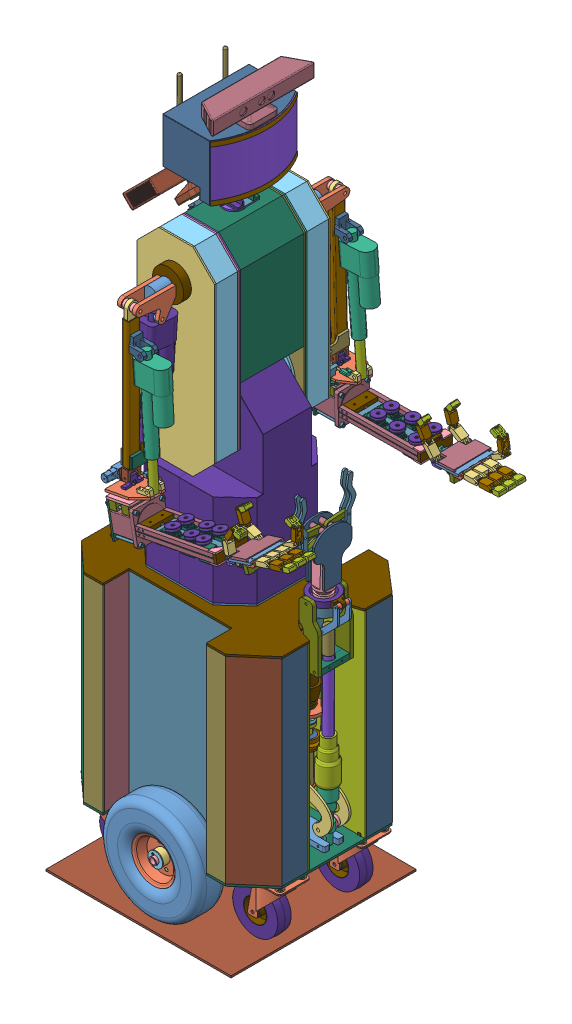
SolidWorks assembly sorbot, configuration По умолчанию. Lengths in mm. (continued)
Mates (geometry in assembly coordinates): (continued)
- Концентричный555: concentric anti-aligned: cylinder of arm.drive.p3-2 through (-20.8275 1162.0905 -207.3595) axis (0 0 -1) radius 6; cylinder of arm.drive.p6-2 through (-20.8275 1162.0905 -222.3595) axis (0 0 1) radius 7
- Заблокировать505: lock: unknown of body.frame.p1-3; unknown of ?
- Заблокировать506: lock: unknown of body.frame.p1-left-1; unknown of ?
- Заблокировать507: lock: unknown of body.frame.p1-3; unknown of ?
- Заблокировать508: lock: unknown of body.frame.p1-3; unknown of arm.drive.p6-1
- Заблокировать510: lock: unknown of ?; unknown of ?
- Концентричный559: concentric anti-aligned: cylinder of arm.drive.p3-2 through (-20.8275 1162.0905 -207.3595) axis (0 0 -1) radius 6; cylinder of m14.nut-1 through (-20.8275 1162.0905 -128.9852) axis (0 0 1) radius 7
- Совпадение1034: coincident anti-aligned: plane of arm.drive.p7-2 through (-42.4721 1162.0905 -109.4852) normal (0 1 0); plane of arm.drive.p7-3 through (-42.4721 1162.0905 -137.4852) normal (0 -1 0)
- Совпадение1035: coincident aligned: plane of arm.drive.p7-2 through (12.3724 1162.0905 -109.4852) normal (0 0 1); plane of arm.drive.p7-3 through (12.3724 1162.0905 -109.4852) normal (0 0 1)
- Совпадение1036: coincident aligned: plane of arm.drive.p7-2 through (-42.4721 1162.0905 -137.4852) normal (-1 0 0); plane of arm.drive.p7-3 through (-42.4721 1162.0905 -109.4852) normal (-1 0 0)
- Концентричный560: concentric anti-aligned: cylinder of arm.drive.p2-pair-1 through (10.8018 1164.5905 -123.4852) axis (0 -1 0) radius 2.5; cylinder of arm.drive.p7-3 through (10.8018 1162.0905 -123.4852) axis (0 1 0) radius 2.5
- Совпадение1038: coincident anti-aligned: plane of m14.nut-1 through (-8.1258 1162.0905 -128.9852) normal (0 0 -1); plane of arm.drive.p7-3 through (-33.7738 1162.0905 -128.9852) normal (0 0 1)
- Заблокировать511: lock: unknown of ?; unknown of ?
- Совпадение1040: coincident anti-aligned: plane of arm.drive.p7-4 through (-9.0342 1232.7974 -150.3) normal (0 1 0); plane of m14.nut-2 through (-2.5764 1232.7974 -139.8) normal (0 -1 0)
- Совпадение1041: coincident anti-aligned: plane of m14.nut-2 through (-2.5764 1254.7974 -150.3) normal (0 0 -1); plane of arm.drive.p7-4 through (-9.0341 1243.9206 -150.3) normal (0 0 1)
- Совпадение1042: coincident: plane of arm.drive.p7-4 through (16.4762 1232.7974 -150.3) normal (-1 0 0); line of m14.nut-2 through (16.4762 1243.7974 -140.8) axis (0 0 -1)
- Заблокировать512: lock: unknown of ?; unknown of ?
- Концентричный562: concentric anti-aligned: cylinder of m14.nut-2 through (3.7745 1243.7974 -139.8) axis (0 0 -1) radius 7; cylinder of arm.drive.p3-1 through (3.7745 1243.7974 -65.7442) axis (0 0 1) radius 6
- Совпадение1043: coincident anti-aligned: plane of arm.drive.p7-5 through (-17.7325 1243.9206 -159.3) normal (0 -1 0); plane of arm.drive.p7-4 through (-17.7325 1243.9206 -131.3) normal (0 1 0)
- Концентричный563: concentric anti-aligned: cylinder of arm.drive.p7-4 through (35.5414 1243.9206 -145.3) axis (0 -1 0) radius 2.5; cylinder of arm.drive.p7-5 through (35.5414 1243.9206 -145.3) axis (0 1 0) radius 2.5
- Совпадение1045: coincident aligned: plane of arm.drive.p7-4 through (-17.7325 1243.9206 -159.3) normal (-1 0 0); plane of arm.drive.p7-5 through (-17.7325 1243.9206 -131.3) normal (-1 0 0)
- Совпадение1046: coincident aligned: plane of arm.drive.p7-4 through (37.112 1243.9206 -131.3) normal (0 0 1); plane of arm.drive.p7-5 through (37.112 1243.9206 -131.3) normal (0 0 1)
- Концентричный564: concentric anti-aligned: cylinder of arm.drive.p2-1 through (35.5414 1246.2974 -145.3) axis (0 -1 0) radius 2.5; cylinder of arm.drive.p7-5 through (35.5414 1243.9206 -145.3) axis (0 1 0) radius 2.5
- Совпадение1047: coincident anti-aligned: plane of body.frame.p4-4 through (-117.3772 1436.2936 -230.3595) normal (0 0 -1); plane of arm.drive.p1.m1-1 through (28.6519 1174.5905 -230.3595) normal (0 0 1)
- Совпадение1048: coincident anti-aligned: plane of body.frame.p4-4 through (-117.3772 1436.2936 -230.3595) normal (0 0 -1); plane of arm.drive.p1.m1-2 through (28.6519 1159.5905 -230.3595) normal (0 0 1)
- Параллельность203: parallel anti-aligned: plane of arm.drive.p1.m1-1 through (28.6519 1164.5905 -234.3595) normal (0 -1 0); plane of arm.drive.p1.m1-2 through (28.6519 1159.5905 -234.3595) normal (0 1 0)
- Совпадение1051: coincident anti-aligned: plane of ? through (48.6519 1164.5905 -237.3595) normal (0 1 0); plane of arm.drive.p1.m1-1 through (28.6519 1164.5905 -234.3595) normal (0 -1 0)
- Совпадение1052: coincident aligned: plane of arm.drive.p1.m1-1 through (68.6519 1174.5904 -230.3595) normal (1 0 0); plane of arm.drive.p1.m1-2 through (68.6519 1159.5904 -230.3595) normal (1 0 0)
- Совпадение1053: coincident anti-aligned: plane of ? through (48.6519 1159.5905 -237.3595) normal (0 -1 0); plane of arm.drive.p1.m1-2 through (28.6519 1159.5905 -234.3595) normal (0 1 0)
- Заблокировать513: lock: unknown of ?; unknown of ?
- Заблокировать514: lock: unknown of ?; unknown of ?
- Концентричный565: concentric aligned: cylinder of ? through (48.6519 1164.5905 -237.3595) axis (0 -1 0) radius 2.5; cylinder of arm.drive.p1.m1-2 through (48.6519 1159.5905 -237.3595) axis (0 -1 0) radius 2.5
- Концентричный566: concentric anti-aligned: cylinder of shoulder.bearing.housing-3 through (-12.6499 1335.3853 -313.3595) axis (0 0 1) radius 15.5; cylinder of body.frame.p4.external-1 through (-12.6499 1335.3853 -288.3595) axis (0 0 -1) radius 21
- Заблокировать516: lock: unknown of ?; unknown of ?
- Заблокировать517: lock: unknown of ?; unknown of ?
- Заблокировать518: lock: unknown of ?; unknown of ?
- Концентричный567: concentric aligned: cylinder of shoulder.bearing.housing-1 through (-12.7629 1335.3853 40.2558) axis (0 0 -1) radius 15.5; cylinder of body.frame.p4.external-2 through (-12.7629 1335.3853 19.2558) axis (0 0 -1) radius 21
- Заблокировать520: lock: unknown of body.frame.p5-1; unknown of body.frame.p4.external-2
- Заблокировать522: lock: unknown of arm.lift.actuator.fixture.p3-1; unknown of body.frame.p4.external-2
- Заблокировать523: lock: unknown of shoulder.bearing.housing-1; unknown of body.frame.p4.external-2
- Заблокировать524: lock: unknown of arm.lift.actuator.fixture.p2-1; unknown of arm.lift.actuator.fixture.p3-1
- Совпадение1061: coincident anti-aligned: plane of ? through (45.4163 1246.2974 -35.7442) normal (0 1 0); plane of arm.drive.p1.m1-4 through (65.4163 1246.2974 -38.7442) normal (0 -1 0)
- Совпадение1064: coincident aligned: plane of arm.drive.p1.m1-3 through (65.4163 1241.2974 -42.7442) normal (1 0 0); plane of arm.drive.p1.m1-4 through (65.4163 1256.2974 -42.7442) normal (1 0 0)
- Совпадение1065: coincident anti-aligned: plane of ? through (45.4163 1241.2974 -35.7442) normal (0 -1 0); plane of arm.drive.p1.m1-3 through (65.4163 1241.2974 -38.7442) normal (0 1 0)
- Концентричный568: concentric aligned: cylinder of ? through (45.4163 1246.2974 -35.7442) axis (0 -1 0) radius 2.5; cylinder of arm.drive.p1.m1-4 through (45.4163 1256.2974 -35.7442) axis (0 -1 0) radius 2.5
- Концентричный569: concentric anti-aligned: cylinder of shoulder.bearing.housing-2 through (-12.4903 1335.516 -67.7442) axis (0 0 1) radius 15.5; cylinder of body.frame.p4.right-1 through (-12.4903 1335.516 -42.7442) axis (0 0 -1) radius 12.5
- Заблокировать527: lock: unknown of arm.lift.actuator.fixture.p3-2; unknown of body.frame.p4.right-1
- Заблокировать528: lock: unknown of shoulder.bearing.housing-2; unknown of body.frame.p4.right-1
- Заблокировать529: lock: unknown of body.frame.p5-1; unknown of body.frame.p4.right-1
- Заблокировать530: lock: unknown of arm.drive.p1.m1-4; unknown of body.frame.p4.right-1
- Заблокировать531: lock: unknown of arm.drive.p1.m1-3; unknown of body.frame.p4.right-1
- Совпадение1067: coincident anti-aligned: plane of body.frame.p1-3 through (92.5097 1436.2936 -46.7442) normal (0 0 1); plane of body.frame.p4.right-1 through (-117.4903 1436.2936 -46.7442) normal (0 0 -1)
- Совпадение1026: coincident anti-aligned: plane of body.frame.p4-4 through (-117.3772 1436.2936 -226.3595) normal (0 0 1); plane of body.frame.p1-left-1 through (92.5148 1436.2936 -226.3595) normal (0 0 -1)
- Концентричный570: concentric aligned: cylinder of arm.drive.motor-1 through (-20.8275 1162.0905 -80.2442) axis (0 0 1) radius 8; cylinder of arm.drive.p8-1 through (-20.8275 1162.0905 -80.2442) axis (0 0 1) radius 8
- Совпадение1069: coincident anti-aligned: plane of arm.drive.motor-1 through (-20.8275 1162.0905 -72.7442) normal (0 0 -1); plane of arm.drive.p8-1 through (-20.8275 1162.0905 -72.7442) normal (0 0 1)
- Концентричный571: concentric aligned: cylinder of arm.drive.motor.pair-1 through (3.7745 1243.7974 -192.8595) axis (0 0 -1) radius 8; cylinder of arm.drive.p8-2 through (3.7745 1243.7974 -192.8595) axis (0 0 -1) radius 8
- Совпадение1070: coincident anti-aligned: plane of arm.drive.motor.pair-1 through (3.7745 1243.7974 -200.3595) normal (0 0 1); plane of arm.drive.p8-2 through (3.7745 1243.7974 -200.3595) normal (0 0 -1)
- Концентричный572: concentric aligned: cylinder of man1.drive1-1 through (-119.3768 773.978 -141.6211) axis (0 -1 0) radius 6; cylinder of tilt.thread.rod.fixture.2-1 through (-119.3768 819.5591 -141.6211) axis (0 -1 0) radius 12
- Совпадение1071: coincident anti-aligned: plane of turret.table-1 through (-20.0648 612.7934 -360.2969) normal (0 1 0); plane of body.tilit.planetary.drive.fixture.p1-1 through (-119.3768 612.7934 -141.6211) normal (0 -1 0)
- Концентричный573: concentric aligned: cylinder of man1.drive1-1 through (-119.3768 703.728 -141.6211) axis (0 -1 0) radius 19; cylinder of body.tilit.planetary.drive.fixture.p1-1 through (-119.3768 622.7934 -141.6211) axis (0 -1 0) radius 42.5
- Заблокировать532: lock: unknown of ?; unknown of ?
- Совпадение1072: coincident anti-aligned: plane of body.tilit.planetary.drive.fixture.p1-1 through (-119.3768 622.7934 -141.6211) normal (0 1 0); plane of body.tilit.planetary.drive.fixture.p2-1 through (-119.3768 622.7934 -141.6211) normal (0 -1 0)
- Концентричный575: concentric aligned: cylinder of body.tilit.planetary.drive.fixture.p1-1 through (-119.3768 622.7934 -141.6211) axis (0 -1 0) radius 42.5; cylinder of body.tilit.planetary.drive.fixture.p2-1 through (-119.3768 626.7934 -141.6211) axis (0 -1 0) radius 42.5
- Концентричный577: concentric aligned: cylinder of man1.drive1-1 through (-119.3768 773.978 -141.6211) axis (0 -1 0) radius 6; cylinder of tilt.thread.rod.fixture.2-2 through (-119.3768 792.5591 -141.6211) axis (0 -1 0) radius 8
- Совпадение1073: coincident anti-aligned: plane of tilt.thread.rod.fixture.2-1 through (-119.3768 793.5591 -141.6211) normal (0 -1 0); plane of tilt.thread.rod.fixture.2-2 through (-119.3768 793.5591 -141.6211) normal (0 1 0)
- Концентричный578: concentric aligned: cylinder of man1.drive1-1 through (-119.3768 703.728 -141.6211) axis (0 -1 0) radius 19; cylinder of body.tilit.planetary.drive.fixture.p3-1 through (-119.3768 703.728 -141.6211) axis (0 -1 0) radius 19
- Совпадение1074: coincident anti-aligned: plane of man1.drive1-1 through (-119.3768 703.728 -141.6211) normal (0 -1 0); plane of body.tilit.planetary.drive.fixture.p3-1 through (-119.3768 703.728 -141.6211) normal (0 1 0)
- Концентричный579: concentric aligned: cylinder of man1.drive1-1 through (-119.3768 761.728 -141.6211) axis (0 -1 0) radius 14.75; cylinder of body.tilit.planetary.drive.fixture.p4-1 through (-119.3768 762.9526 -141.6211) axis (0 -1 0) radius 14.8
- Заблокировать533: lock: unknown of ?; unknown of ?
- Концентричный580: concentric anti-aligned: cylinder of body.tilit.planetary.drive.fixture.p3-1 through (-148.8664 695.728 -141.6211) axis (0 1 0) radius 2.5; cylinder of body.tilit.planetary.drive.fixture.p5-1 through (-148.8664 769.7934 -141.6211) axis (0 -1 0) radius 2.5
- Совпадение1076: coincident aligned: plane of body.tilit.planetary.drive.fixture.p1-1 through (-119.3768 612.7934 -141.6211) normal (0 -1 0); plane of body.tilit.planetary.drive.fixture.p5-1 through (-148.8664 612.7934 -141.6211) normal (0 -1 0)
- Совпадение1077: coincident anti-aligned: plane of body.tilit.planetary.drive.fixture.p1-1 through (-148.8664 618.7934 -141.6211) normal (0 -1 0); plane of m6.nut-13 through (-148.8664 618.7934 -135.8476) normal (0 1 0)
- Концентричный581: concentric aligned: cylinder of body.tilit.planetary.drive.fixture.p5-1 through (-148.8664 769.7934 -141.6211) axis (0 -1 0) radius 2.5; cylinder of m6.nut-13 through (-148.8664 618.7934 -141.6211) axis (0 -1 0) radius 3
- Концентричный582: concentric aligned: cylinder of body.tilit.planetary.drive.fixture.p1-1 through (-119.3768 624.7934 -112.1315) axis (0 -1 0) radius 2.5; cylinder of body.tilit.planetary.drive.fixture.p5-3 through (-119.3768 769.7934 -112.1315) axis (0 -1 0) radius 2.5
- Концентричный583: concentric aligned: cylinder of body.tilit.planetary.drive.fixture.p1-1 through (-89.8872 624.7934 -141.6211) axis (0 -1 0) radius 2.5; cylinder of body.tilit.planetary.drive.fixture.p5-2 through (-89.8872 769.7934 -141.6211) axis (0 -1 0) radius 2.5
- Концентричный584: concentric aligned: cylinder of body.tilit.planetary.drive.fixture.p1-1 through (-119.3768 624.7934 -171.1107) axis (0 -1 0) radius 2.5; cylinder of body.tilit.planetary.drive.fixture.p5-4 through (-119.3768 769.7934 -171.1107) axis (0 -1 0) radius 2.5
- Совпадение1078: coincident aligned: plane of body.tilit.planetary.drive.fixture.p1-1 through (-119.3768 612.7934 -141.6211) normal (0 -1 0); plane of body.tilit.planetary.drive.fixture.p5-4 through (-119.3768 612.7934 -171.1107) normal (0 -1 0)
- Совпадение1079: coincident aligned: plane of body.tilit.planetary.drive.fixture.p1-1 through (-119.3768 612.7934 -141.6211) normal (0 -1 0); plane of body.tilit.planetary.drive.fixture.p5-3 through (-119.3768 612.7934 -112.1315) normal (0 -1 0)
- Совпадение1080: coincident aligned: plane of body.tilit.planetary.drive.fixture.p1-1 through (-119.3768 612.7934 -141.6211) normal (0 -1 0); plane of body.tilit.planetary.drive.fixture.p5-2 through (-89.8872 612.7934 -141.6211) normal (0 -1 0)
- Концентричный585: concentric aligned: cylinder of body.tilit.planetary.drive.fixture.p5-4 through (-119.3768 769.7934 -171.1107) axis (0 -1 0) radius 2.5; cylinder of m6.nut-15 through (-119.3768 618.7934 -171.1107) axis (0 -1 0) radius 3
- Концентричный586: concentric aligned: cylinder of body.tilit.planetary.drive.fixture.p5-2 through (-89.8872 769.7934 -141.6211) axis (0 -1 0) radius 2.5; cylinder of m6.nut-14 through (-89.8872 618.7934 -141.6211) axis (0 -1 0) radius 3
- Концентричный587: concentric aligned: cylinder of body.tilit.planetary.drive.fixture.p5-3 through (-119.3768 769.7934 -112.1315) axis (0 -1 0) radius 2.5; cylinder of m6.nut-16 through (-119.3768 618.7934 -112.1315) axis (0 -1 0) radius 3
- Совпадение1081: coincident anti-aligned: plane of body.tilit.planetary.drive.fixture.p1-1 through (-119.3768 618.7934 -112.1315) normal (0 -1 0); plane of m6.nut-16 through (-113.8446 618.7934 -113.783) normal (0 1 0)
- Совпадение1082: coincident anti-aligned: plane of body.tilit.planetary.drive.fixture.p1-1 through (-89.8872 618.7934 -141.6211) normal (0 -1 0); plane of m6.nut-14 through (-89.8872 618.7934 -135.8476) normal (0 1 0)
- Совпадение1083: coincident anti-aligned: plane of body.tilit.planetary.drive.fixture.p1-1 through (-119.3768 618.7934 -171.1107) normal (0 -1 0); plane of m6.nut-15 through (-114.7531 618.7934 -167.6531) normal (0 1 0)
- Совпадение1084: coincident anti-aligned: plane of body.tilit.planetary.drive.fixture.p4-1 through (-119.3768 762.9526 -141.6211) normal (0 1 0); plane of m6.nut-17 through (-122.5346 762.9526 -107.2981) normal (0 -1 0)
- Совпадение1085: coincident anti-aligned: plane of body.tilit.planetary.drive.fixture.p4-1 through (-119.3768 762.9526 -141.6211) normal (0 1 0); plane of m6.nut-18 through (-93.045 762.9526 -136.7877) normal (0 -1 0)
- Совпадение1086: coincident anti-aligned: plane of m6.nut-19 through (-122.5346 762.9526 -166.2773) normal (0 -1 0); plane of body.tilit.planetary.drive.fixture.p4-1 through (-119.3768 762.9526 -141.6211) normal (0 1 0)
- Совпадение1087: coincident anti-aligned: plane of body.tilit.planetary.drive.fixture.p4-1 through (-119.3768 762.9526 -141.6211) normal (0 1 0); plane of m6.nut-20 through (-152.0242 762.9526 -136.7877) normal (0 -1 0)
- Концентричный588: concentric anti-aligned: cylinder of body.tilit.planetary.drive.fixture.p5-1 through (-148.8664 769.7934 -141.6211) axis (0 -1 0) radius 2.5; cylinder of m6.nut-20 through (-148.8664 762.9526 -141.6211) axis (0 1 0) radius 3
- Концентричный589: concentric anti-aligned: cylinder of body.tilit.planetary.drive.fixture.p5-4 through (-119.3768 769.7934 -171.1107) axis (0 -1 0) radius 2.5; cylinder of m6.nut-19 through (-119.3768 762.9526 -171.1107) axis (0 1 0) radius 3
- Концентричный590: concentric anti-aligned: cylinder of body.tilit.planetary.drive.fixture.p5-2 through (-89.8872 769.7934 -141.6211) axis (0 -1 0) radius 2.5; cylinder of m6.nut-18 through (-89.8872 762.9526 -141.6211) axis (0 1 0) radius 3
- Концентричный591: concentric anti-aligned: cylinder of body.tilit.planetary.drive.fixture.p5-3 through (-119.3768 769.7934 -112.1315) axis (0 -1 0) radius 2.5; cylinder of m6.nut-17 through (-119.3768 762.9526 -112.1315) axis (0 1 0) radius 3
- Касательный36: tangent anti-aligned: cylinder of shoulder.p6-2 through (-12.6483 1335.4904 4.6679) axis (0 0 1) radius 19.94; plane of m6.nut-21 through (-29.5996 1324.99 15.6749) normal (0.850111 0.526603 0)
- Концентричный592: concentric aligned: cylinder of shoulder.p6-2 through (-72.9636 1298.128 9.9014) axis (0.850111 0.526603 0) radius 3; cylinder of m6.nut-21 through (-34.2752 1322.0936 9.9014) axis (0.850111 0.526603 0) radius 3
- Концентричный593: concentric aligned: cylinder of m6.6.50mm-1 through (-38.2027 1319.6607 9.9014) axis (0.850111 0.526603 0) radius 3; cylinder of shoulder.p6-2 through (-72.9636 1298.128 9.9014) axis (0.850111 0.526603 0) radius 3
- Касательный37: tangent anti-aligned: cylinder of shoulder.p6-2 through (-12.6483 1335.4904 4.6679) axis (0 0 1) radius 19.94; plane of m6.6.50mm-1 through (4.3029 1345.9909 9.9014) normal (-0.850111 -0.526603 0)
- Концентричный594: concentric anti-aligned: cylinder of shoulder.p6-2 through (-35.3987 1340.8364 -1.3321) axis (0 0 1) radius 2; cylinder of m4.nut-1 through (-35.3987 1340.8364 9.6679) axis (0 0 -1) radius 2
- Совпадение1088: coincident anti-aligned: plane of shoulder.p6-2 through (-12.6483 1335.4904 4.6679) normal (0 0 1); plane of m4.nut-1 through (-35.3987 1336.8758 4.6679) normal (0 0 -1)
- Концентричный595: concentric anti-aligned: cylinder of shoulder.p4-2 through (-12.6483 1335.4904 0.2558) axis (0 0 -1) radius 15; cylinder of shoulder.p6-2 through (-12.6483 1335.4904 -1.3321) axis (0 0 1) radius 15
- Совпадение1089: coincident anti-aligned: plane of arm.lift.actuator.fixture.p3-2 through (-88.5767 993.1387 -35.7442) normal (0 0 1); plane of m4.nut-2 through (-103.2224 993.9386 -35.7442) normal (0 0 -1)
- Концентричный596: concentric anti-aligned: cylinder of arm.lift.actuator.fixture.p3-2 through (-103.2224 997.8992 -42.7442) axis (0 0 1) radius 2; cylinder of m4.nut-2 through (-103.2224 997.8992 -30.7442) axis (0 0 -1) radius 2
- Заблокировать534: lock: unknown of ?; unknown of ?
- Заблокировать535: lock: unknown of ?; unknown of ?
- Концентричный598: concentric aligned: cylinder of forearm.rotate.p9-1 through (-12.6985 939.7014 123.1926) axis (0 0 1) radius 2.5; cylinder of arm.rotate.p8-1 through (-12.6985 939.7014 130.5417) axis (0 0 1) radius 2.5
- Совпадение1090: coincident: plane of forearm.rotate.p9-1 through (-2.9289 953.7014 150.5417) normal (0 0 -1); plane of ? through (-12.4887 947.5088 150.5417) normal (0 0 1)
- Параллельность206: parallel aligned: plane of arm.p1.m-1 through (-18.263 964.7884 156.4102) normal (0 0 1); plane of body.frame.p4.external-2 through (-117.7515 1436.1748 19.2558) normal (0 0 1)
- Совпадение1094: coincident aligned: plane of lower.arm.p2-1 through (42.4949 859.0482 173.2746) normal (-0.982605 -0.185706 0); plane of arm.rotate.p9-1 through (40.6378 868.8743 172.7746) normal (-0.982605 -0.185706 0)
- Совпадение1095: coincident anti-aligned: plane of lower.arm.p3-1 through (252.7724 898.7894 97.2746) normal (0.982605 0.185706 0); plane of lower.arm.p8-2 through (256.6003 878.5354 183.2746) normal (-0.982605 -0.185706 0)
- Расстояние23: distance = 14 mm: plane of ? through (184.7654 908.6895 173.2746) normal (-0.9762 -0.216874 0); plane of ? through (171.0986 905.6533 150.8374) normal (0.9762 0.216874 0)
- Совпадение1100: coincident anti-aligned: plane of lower.arm.p2-3 through (250.9153 908.6154 107.2746) normal (0 0 1); plane of HS-311 Hitec Standard Servo and Horn-4/HS-311 Hitec Standard Servo-1 through (199.6563 888.7508 107.2746) normal (0 0 -1)
- Расстояние24: distance = 14 mm anti-aligned: plane of ? through (171.0986 905.6533 109.8374) normal (0.9762 0.216874 0); plane of ? through (184.7654 908.6895 127.5946) normal (-0.9762 -0.216874 0)
- Заблокировать539: lock: unknown of ?; unknown of ?
- Заблокировать540: lock: plane of ?; plane of arm.rotate-1/SY85STH65-2808A-1
- Расстояние25: distance = 0.5 mm anti-aligned: plane of lower.arm.p3-1 through (42.4949 859.0482 146.4722) normal (-0.982605 -0.185706 0); plane of arm.rotate-1/SY85STH65-2808A-1 through (42.1893 857.9727 140.2746) normal (0.982605 0.185706 0)
- Заблокировать541: lock: unknown of ?; unknown of ?
- Совпадение1112: coincident anti-aligned: plane of lower.arm.p3-1 through (42.4949 859.0482 134.0356) normal (-0.185706 0.982605 0); plane of arm.rotate.p9-1 through (42.4949 859.0482 107.7746) normal (0.185706 -0.982605 0)
- Совпадение1114: coincident anti-aligned: plane of lower.arm.p3-1 through (42.8663 857.083 134.0356) normal (0.185706 -0.982605 0); plane of arm.rotate.p9-2 through (72.3444 862.6542 107.7746) normal (-0.185706 0.982605 0)
- Концентричный603: concentric anti-aligned: cylinder of arm.rotate-1/SY85STH65-2808A-1 through (71.6674 863.5439 140.2746) axis (-0.982605 -0.185706 0) radius 6; cylinder of arm.rotate.p9-1 through (42.6806 858.0656 140.2746) axis (0.982605 0.185706 0) radius 6
- Концентричный604: concentric aligned: cylinder of arm.rotate-1/SY85STH65-2808A-1 through (71.6674 863.5439 140.2746) axis (-0.982605 -0.185706 0) radius 6; cylinder of arm.rotate.p9-2 through (72.1587 863.6368 140.2746) axis (-0.982605 -0.185706 0) radius 6
- Совпадение1115: coincident anti-aligned: plane of lower.arm.p2-1 through (252.7724 898.7894 173.2746) normal (0.982605 0.185706 0); plane of lower.arm.p8-2 through (256.6003 878.5354 183.2746) normal (-0.982605 -0.185706 0)
- Расстояние26: distance = 120 mm aligned: unknown of ?; unknown of ?
- Расстояние27: distance = 30 mm aligned: unknown of ?; unknown of ?
- Совпадение1119: coincident anti-aligned: plane of arm.rotate.p8-1 through (-3.0887 921.1635 130.5417) normal (0.185706 -0.982605 0); plane of arm.rotate.p6-1 through (-41.1593 913.9684 182.7746) normal (-0.185706 0.982605 0)
- Совпадение1120: coincident anti-aligned: plane of ? through (-46.5956 921.7238 182.7746) normal (0.060639 0.99816 0); plane of arm.rotate.p7-1 through (19.283 917.7216 160.2746) normal (-0.060639 -0.99816 0)
- Заблокировать542: lock: unknown of ?; unknown of ?
- Совпадение1122: coincident aligned: plane of ?; plane of ?
- Заблокировать543: lock: unknown of ?; unknown of ?
- Совпадение1123: coincident anti-aligned: plane of ? through (-46.5956 921.7238 182.7746) normal (0.060639 0.99816 0); plane of ? through (19.283 917.7216 130.2746) normal (-0.060639 -0.99816 0)
- Касательный40: tangent anti-aligned: plane of arm.rotate.p7-2 through (56.0951 948.6321 130.2746) normal (0 0 1); cylinder of arm.actuator100mm.p2-1 through (49.2564 930.6158 140.2746) axis (-0.061067 0.998134 0) radius 10
- Концентричный606: concentric aligned: cylinder of arm.actuator100mm.p2-1 through (48.7373 939.0999 165.2746) axis (0 0 -1) radius 4; cylinder of arm.rotate.p7-2 through (48.7373 939.0999 130.2746) axis (0 0 -1) radius 4
- Совпадение1124: coincident aligned: plane of ? through (55.2167 915.5386 97.7746) normal (0.99816 -0.060639 0); plane of ? through (57.0359 945.4834 120.2746) normal (0.99816 -0.060639 0)
- Заблокировать544: lock: unknown of ?; unknown of ?
- Концентричный607: concentric aligned: cylinder of arm.actuator100mm.p2-1 through (48.7373 939.0999 165.2746) axis (0 0 -1) radius 4; cylinder of arm.rotate.p7-1 through (48.7373 939.0999 160.2746) axis (0 0 -1) radius 4
- Совпадение1125: coincident: plane of arm.rotate-1/arm.rotate.p2-2; plane of arm.rotate.p10-1
- Совпадение1126: coincident: plane of arm.rotate-1/arm.rotate.p1-3; plane of ?
- Совпадение1127: coincident anti-aligned: plane of ?; plane of ?
- Заблокировать545: lock: unknown of ?; unknown of ?
- Расстояние28: distance = 9.5 mm anti-aligned: plane of arm.rotate.p6-1 through (-40.0451 908.0728 182.7746) normal (0.185706 -0.982605 0); plane of arm.rotate.p10-1 through (25.5885 910.8089 182.7746) normal (-0.185706 0.982605 0)
- Касательный41: tangent anti-aligned: unknown of ?; sphere of ?
- Касательный42: tangent anti-aligned: plane of arm.rotate.p10-1 through (25.5885 910.8089 182.7746) normal (-0.185706 0.982605 0); unknown of ?
- Концентричный608: concentric aligned: cylinder of arm.rotate.p10-1 through (-6.3462 904.7735 140.2746) axis (0.185706 -0.982605 0) radius 4; cylinder of arm.elbow.rotate.bearing-1/arm.elbow.rotate.bearing.p1-1 through (-7.6926 911.8974 140.2746) axis (0.185706 -0.982605 0) radius 18.2
- Концентричный609: concentric anti-aligned: cylinder of arm.rotate.p6-1 through (-8.1104 914.1082 140.2746) axis (-0.185706 0.982605 0) radius 4; cylinder of arm.rotate.p10-1 through (-6.3462 904.7735 140.2746) axis (0.185706 -0.982605 0) radius 4
- Совпадение1128: coincident anti-aligned: plane of arm.rotate.p10-1 through (26.7027 904.9133 182.7746) normal (0.185706 -0.982605 0); plane of bolt.m8.short-1 through (-5.232 898.8778 140.2746) normal (-0.185706 0.982605 0)
- Концентричный610: concentric aligned: cylinder of arm.rotate.p10-1 through (-6.3462 904.7735 140.2746) axis (0.185706 -0.982605 0) radius 4; cylinder of bolt.m8.short-1 through (-11.7317 933.269 140.2746) axis (0.185706 -0.982605 0) radius 4
- Концентричный612: concentric aligned: cylinder of ? through (-13.9627 933.3208 140.2746) axis (-0.157334 -0.987545 0) radius 4; cylinder of m8.nut-1 through (-14.9853 926.9018 140.2746) axis (-0.157334 -0.987545 0) radius 4
- Заблокировать547: lock: unknown of ?; unknown of ?
- Совпадение1129: coincident anti-aligned: plane of arm.rotate.p10-1 through (25.5885 910.8089 182.7746) normal (-0.185706 0.982605 0); plane of arm.elbow.rotate.p3-1 through (-6.3462 904.7735 140.2746) normal (0.185706 -0.982605 0)
- Концентричный613: concentric aligned: cylinder of ? through (-7.6926 911.8974 140.2746) axis (0.185706 -0.982605 0) radius 18.2; cylinder of ? through (-8.0176 913.6169 140.2746) axis (0.185706 -0.982605 0) radius 18.2
- Совпадение1130: coincident anti-aligned: plane of arm.rotate.p10-1 through (25.5885 910.8089 182.7746) normal (-0.185706 0.982605 0); plane of arm.elbow.rotate.p4-1 through (-6.3462 904.7735 140.2746) normal (0.185706 -0.982605 0)
- Концентричный614: concentric aligned: cylinder of ? through (-8.0176 913.6169 140.2746) axis (0.185706 -0.982605 0) radius 11; cylinder of ? through (-7.6461 911.6517 140.2746) axis (0.185706 -0.982605 0) radius 11
- Совпадение1140: coincident anti-aligned: plane of ? through (-48.1819 925.1023 182.7746) normal (0.157334 0.987545 0); plane of ? through (-12.3806 919.3985 146.7746) normal (-0.157334 -0.987545 0)
- Заблокировать549: lock: unknown of ?; unknown of ?
- Заблокировать550: lock: unknown of ?; unknown of ?
- Заблокировать551: lock: unknown of ?; unknown of ?
- Заблокировать552: lock: unknown of ?; unknown of ?
- Заблокировать553: lock: unknown of ?; unknown of ?
- Параллельность209: parallel aligned: plane of arm.rotate.p9-1 through (40.6378 868.8743 107.7746) normal (-0.185706 0.982605 0); plane of arm.rotate.p10-1 through (25.5885 910.8089 182.7746) normal (-0.185706 0.982605 0)
- Концентричный615: concentric aligned: cylinder of arm.elbow.rotate.p5-1 through (35.8794 941.7075 114.7746) axis (-0.982605 -0.185706 0) radius 2.5; cylinder of arm.elbow.rotate.p11-1 through (8.5139 936.5356 114.7746) axis (-0.982605 -0.185706 0) radius 2.5
- Концентричный616: concentric anti-aligned: cylinder of arm.rotate.p10-1 through (18.8419 903.4277 105.7746) axis (-0.185706 0.982605 0) radius 2.5; cylinder of arm.elbow.rotate.p12-1 through (16.8919 913.745 105.7746) axis (0.185706 -0.982605 0) radius 2.5
- Совпадение1141: coincident anti-aligned: plane of arm.rotate.p10-1 through (25.5885 910.8089 182.7746) normal (-0.185706 0.982605 0); plane of arm.elbow.rotate.p12-1 through (8.8842 907.6519 93.7746) normal (0.185706 -0.982605 0)
- Параллельность207: parallel aligned: plane of arm.rotate.p6-1 through (59.0664 932.9105 182.7746) normal (0 0 1); plane of arm.rotate.p10-1 through (-38.2809 898.738 182.7746) normal (0 0 1)
- Концентричный617: concentric aligned: cylinder of arm.elbow.rotate.p11-1 through (4.2377 932.2373 93.7746) axis (0.185706 -0.982605 0) radius 2.5; cylinder of arm.elbow.rotate.p12-1 through (8.0485 912.0737 93.7746) axis (0.185706 -0.982605 0) radius 2.5
- Концентричный619: concentric anti-aligned: cylinder of arm.elbow.rotate.p5-1 through (35.8794 941.7075 114.7746) axis (-0.982605 -0.185706 0) radius 2.5; cylinder of arm.elbow.rotate.p13-1 through (-38.1599 927.7145 114.7746) axis (0.982605 0.185706 0) radius 2.5
- Совпадение1142: coincident anti-aligned: plane of arm.elbow.rotate.p1-1 through (-37.3429 925.2763 117.1746) normal (0 0 1); plane of arm.elbow.rotate.p13-1 through (-37.6868 925.2113 117.1746) normal (0 0 -1)
- Совпадение1144: coincident anti-aligned: plane of arm.elbow.rotate.p1-1 through (-43.0729 926.786 114.7746) normal (0.982605 0.185706 0); plane of arm.elbow.rotate.p13-1 through (-43.0729 926.786 114.7746) normal (-0.982605 -0.185706 0)
- Концентричный620: concentric anti-aligned: cylinder of arm.elbow.rotate.p13-1 through (-43.0729 926.786 114.7746) axis (0.982605 0.185706 0) radius 4.5; cylinder of arm.elbow.rotate.p14-1 through (-31.773 928.9216 114.7746) axis (-0.982605 -0.185706 0) radius 4.5
- Совпадение1145: coincident anti-aligned: plane of arm.rotate.p11-1 through (-39.1941 914.3398 97.7746) normal (0.982605 0.185706 0); plane of arm.elbow.rotate.p14-1 through (-41.599 927.0645 114.7746) normal (-0.982605 -0.185706 0)
- Параллельность211: parallel aligned: plane of ? through (240.557 838.2014 183.2746) normal (0 0 1); plane of ? through (42.857 823.2014 151.7746) normal (0 0 1)
- Расстояние30: distance = 31.5 mm aligned: plane of ? through (240.557 838.2014 183.2746) normal (0 0 1); plane of ? through (42.857 823.2014 151.7746) normal (0 0 1)
- Совпадение1148: coincident anti-aligned: plane of ? through (56.557 838.2014 172.7746) normal (1 0 0); plane of ? through (56.557 838.2014 140.4246) normal (-1 0 0)
- Касательный45: tangent anti-aligned: plane of ? through (26.557 848.2014 134.0356) normal (0 -1 0); cylinder of ? through (70.257 838.2014 140.4246) axis (-1 0 0) radius 10
- Заблокировать556: lock: unknown of ?; unknown of ?
- Заблокировать558: lock: unknown of ?; unknown of ?
- Концентричный624: concentric aligned: cylinder of palm.tilt.p1-1 through (97.1945 857.1737 140.4246) axis (-0.982605 -0.185706 0) radius 1.5; cylinder of palm.lift.p2-2 through (252.4461 886.5153 140.4246) axis (-0.982605 -0.185706 0) radius 2.5
- Совпадение1156: coincident anti-aligned: plane of palm.tilt.p1-1 through (97.1945 857.1737 140.4246) normal (0.982605 0.185706 0); plane of palm.lift.p2-2 through (97.1945 857.1737 140.4246) normal (-0.982605 -0.185706 0)
- Заблокировать559: lock: unknown of ?; unknown of ?
- Заблокировать560: lock: unknown of ?; unknown of ?
- Заблокировать561: lock: unknown of ?; unknown of ?
- Концентричный625: concentric aligned: cylinder of palm.lift.p2-2 through (252.4461 886.5153 140.4246) axis (-0.982605 -0.185706 0) radius 2.5; cylinder of palm.drive.thread.fixture-1 through (254.516 886.9065 140.4246) axis (-0.982605 -0.185706 0) radius 2.5
- Совпадение1157: coincident anti-aligned: plane of lower.arm.p3-1 through (42.8663 857.083 134.0356) normal (0.185706 -0.982605 0); plane of palm.drive.thread.fixture-1 through (245.7807 895.4326 155.4246) normal (-0.185706 0.982605 0)
- Заблокировать562: lock: unknown of ?; unknown of ?
- Заблокировать563: lock: unknown of ?; unknown of ?
- Концентричный626: concentric aligned: cylinder of palm.lift.fixture-1 through (273.752 896.6482 125.2746) axis (0 0 1) radius 3; cylinder of palm.lift.fixture.p2-1 through (273.752 896.6482 125.2746) axis (0 0 1) radius 3
- Совпадение1164: coincident anti-aligned: plane of lower.arm.p3-1 through (42.8663 857.083 134.0356) normal (0.185706 -0.982605 0); plane of PALM.LIFT.THREAD.FIXTURE.P3-1 through (121.2398 871.8951 145.2958) normal (-0.185706 0.982605 0)
- Концентричный627: concentric anti-aligned: cylinder of palm.lift.p2-2 through (252.4461 886.5153 140.4246) axis (-0.982605 -0.185706 0) radius 2.5; cylinder of PALM.LIFT.THREAD.FIXTURE.P3-1 through (123.0968 862.0691 140.4246) axis (0.982605 0.185706 0) radius 2.5
- Заблокировать565: lock: unknown of ?; unknown of ?
- Концентричный628: concentric aligned: cylinder of palm.lift.p2-2 through (252.4461 886.5153 140.4246) axis (-0.982605 -0.185706 0) radius 2.5; cylinder of palm.lift.drive.nut-1 through (183.8748 873.5557 140.4246) axis (-0.982605 -0.185706 0) radius 2.5
- Совпадение1167: coincident anti-aligned: plane of lower.arm.p3-1 through (42.8663 857.083 134.0356) normal (0.185706 -0.982605 0); plane of palm.lift.nut.fixture-1 through (169.2438 880.9676 140.4246) normal (-0.185706 0.982605 0)
- Совпадение1168: coincident anti-aligned: plane of palm.lift.drive.nut-1 through (180.9269 872.9986 140.4246) normal (-0.982605 -0.185706 0); plane of palm.lift.nut.fixture-1 through (184.2697 855.3117 150.4246) normal (0.982605 0.185706 0)
- Концентричный629: concentric aligned: cylinder of palm.lift.nut.fixture-2 through (171.1009 871.1415 140.4246) axis (0.982605 0.185706 0) radius 4.5; cylinder of palm.lift.drive.nut-1 through (171.1009 871.1415 140.4246) axis (0.982605 0.185706 0) radius 4.5
- Совпадение1169: coincident anti-aligned: plane of lower.arm.p3-1 through (42.8663 857.083 134.0356) normal (0.185706 -0.982605 0); plane of palm.lift.nut.fixture-2 through (179.0699 882.8247 140.4246) normal (-0.185706 0.982605 0)
- Совпадение1170: coincident anti-aligned: plane of palm.lift.drive.nut-1 through (180.9269 872.9986 140.4246) normal (-0.982605 -0.185706 0); plane of palm.lift.nut.fixture-2 through (184.2697 855.3117 130.4246) normal (0.982605 0.185706 0)
- Концентричный630: concentric aligned: cylinder of palm.lift.p4-1 through (286.5037 879.7822 140.4246) axis (-0.982605 -0.185706 0) radius 2; cylinder of palm.drive.thread.fixture-1 through (256.9192 874.1909 140.4246) axis (-0.982605 -0.185706 0) radius 2
- Заблокировать566: lock: unknown of ?; unknown of ?
- Совпадение1173: coincident anti-aligned: plane of palm.lift.fixture-1 through (267.539 889.3678 145.2746) normal (0 0 1); plane of palm.lift.fixture.p2-1 through (259.2428 898.2051 145.2746) normal (0 0 -1)
- Концентричный631: concentric aligned: cylinder of palm.lift.p4-1 through (286.5037 879.7822 140.4246) axis (-0.982605 -0.185706 0) radius 2; cylinder of palm.lift.fixture.p6-1 through (286.5037 879.7822 140.4246) axis (-0.982605 -0.185706 0) radius 2
- Совпадение1174: coincident aligned: plane of palm.lift.p4-1 through (286.5037 879.7822 140.4246) normal (0.982605 0.185706 0); plane of palm.lift.fixture.p6-1 through (286.5037 879.7822 140.4246) normal (0.982605 0.185706 0)
- Совпадение1175: coincident anti-aligned: plane of palm.lift.fixture.p6-1 through (295.2792 887.1977 142.4246) normal (0 0 -1); plane of palm.lift.fixture.p7-1 through (292.1321 880.846 142.4246) normal (0 0 1)
- Концентричный632: concentric anti-aligned: cylinder of palm.lift.fixture.p6-1 through (292.1321 880.846 134.4246) axis (0 0 1) radius 2; cylinder of palm.lift.fixture.p7-1 through (292.1321 880.846 142.4246) axis (0 0 -1) radius 2
- Совпадение1181: coincident anti-aligned: plane of palm.fixture.p14-1 through (318.5768 925.7636 155.9704) normal (-0.311571 0.950223 0); plane of m6.washer-1 through (284.4317 914.5677 140.506) normal (0.311571 -0.950223 0)
- Концентричный634: concentric anti-aligned: cylinder of palm.fixture.p14-1 through (286.3011 908.8663 140.506) axis (-0.311571 0.950223 0) radius 3; cylinder of m6.washer-1 through (283.902 916.183 140.506) axis (0.311571 -0.950223 0) radius 3.25
- Концентричный635: concentric aligned: cylinder of palm.lift.fixture.p2-1 through (291.037 894.4229 140.506) axis (-0.311571 0.950223 0) radius 3; cylinder of m6.washer-2 through (290.0088 897.5587 140.506) axis (-0.311571 0.950223 0) radius 3.25
- Концентричный636: concentric aligned: cylinder of palm.fixture.p14-1 through (286.3011 908.8663 140.506) axis (-0.311571 0.950223 0) radius 3; cylinder of palm.lift.fixture.p2-1 through (291.037 894.4229 140.506) axis (-0.311571 0.950223 0) radius 3
- Совпадение1184: coincident anti-aligned: plane of palm.lift.fixture.p2-1 through (281.0507 896.4104 125.2746) normal (0.311571 -0.950223 0); plane of m6.washer-2 through (289.4791 899.1741 140.506) normal (-0.311571 0.950223 0)
- Концентричный637: concentric anti-aligned: cylinder of palm.lift.fixture.p2-1 through (291.037 894.4229 140.506) axis (-0.311571 0.950223 0) radius 3; cylinder of m6.washer-3 through (286.3011 908.8663 140.506) axis (0.311571 -0.950223 0) radius 3.25
- Совпадение1185: coincident anti-aligned: plane of palm.lift.fixture.p2-1 through (266.9997 900.7485 125.2746) normal (-0.311571 0.950223 0); plane of m6.washer-3 through (286.8308 907.251 140.506) normal (0.311571 -0.950223 0)
- Совпадение1186: coincident anti-aligned: plane of palm.fixture.p14-1 through (320.4462 920.0622 155.9704) normal (0.311571 -0.950223 0); plane of m6.washer-3 through (286.3011 908.8663 140.506) normal (-0.311571 0.950223 0)
- Заблокировать567: lock: unknown of ?; unknown of ?
- Концентричный639: concentric aligned: cylinder of palm.lift.fixture.p7-1 through (305.2733 893.1467 142.4246) axis (0 0 -1) radius 2; cylinder of palm.lift.on-palm.fixture-2 through (305.2733 893.1467 153.2746) axis (0 0 -1) radius 2
- Концентричный640: concentric aligned: cylinder of palm.drive.thread.fixture.p2-2 through (326.1771 915.9699 145.3733) axis (-0.012247 -0.004016 0.999917) radius 1.5; cylinder of palm.lift.p1-1 through (326.1091 915.9476 150.9228) axis (-0.012247 -0.004016 0.999917) radius 1.5
- Заблокировать569: lock: unknown of ?; unknown of ?
- Заблокировать570: lock: unknown of ?; unknown of ?
- Совпадение1192: coincident anti-aligned: plane of palm.tilit.p8-1 through (326.1771 915.9699 145.3733) normal (-0.012247 -0.004016 0.999917); plane of palm.drive.thread.fixture.p2-2 through (326.1771 915.9699 145.3733) normal (0.012247 0.004016 -0.999917)
- Концентричный641: concentric anti-aligned: cylinder of palm.drive.thread.fixture.p2-2 through (326.1771 915.9699 145.3733) axis (0.012247 0.004016 -0.999917) radius 2.5; cylinder of palm.tilit.p8-1 through (326.8752 916.1988 88.378) axis (-0.012247 -0.004016 0.999917) radius 2.5
- Совпадение1193: coincident anti-aligned: plane of palm.lift.p1-1 through (325.9934 915.9097 160.372) normal (0.012247 0.004016 -0.999917); plane of palm.drive.thread.fixture.p2-2 through (325.9934 915.9097 160.372) normal (-0.012247 -0.004016 0.999917)
- Совпадение1194: coincident anti-aligned: plane of palm.tilit.p9-1 through (340.8052 933.0521 97.267) normal (-0.311571 0.950223 0); plane of palm.p1-3 through (364.9952 940.9838 91.5947) normal (0.311571 -0.950223 0)
- Совпадение1195: coincident aligned: plane of palm.p1-3 through (291.8649 923.3193 90.628) normal (0.012247 0.004016 -0.999917); plane of palm.tilit.p9-1 through (342.4366 928.3251 91.2675) normal (0.012247 0.004016 -0.999917)
- Совпадение1196: coincident anti-aligned: plane of palm.lift.on-palm.fixture-2 through (305.7565 904.5113 133.5583) normal (0.950223 0.311571 0); plane of palm.tilit.p10-1 through (305.7565 904.5113 153.2746) normal (-0.950223 -0.311571 0)
- Совпадение1197: coincident aligned: plane of palm.lift.on-palm.fixture-2 through (303.1082 912.5882 153.2746) normal (0 0 1); plane of palm.tilit.p10-1 through (317.3615 917.2617 153.2746) normal (0 0 1)
- Совпадение1198: coincident aligned: plane of palm.lift.on-palm.fixture-2 through (305.7565 904.5113 146.9909) normal (0.311571 -0.950223 0); plane of palm.tilit.p10-1 through (320.0099 909.1848 153.2746) normal (0.311571 -0.950223 0)
- Концентричный642: concentric anti-aligned: cylinder of palm.tilit.p8-1 through (326.8752 916.1988 88.378) axis (-0.012247 -0.004016 0.999917) radius 2.5; cylinder of palm.tilit.p11-1 through (326.4209 916.0499 125.4635) axis (0.012247 0.004016 -0.999917) radius 2.5
- Параллельность212: parallel aligned: plane of palm.tilit.p10-1 through (320.0099 909.1848 153.2746) normal (0.311571 -0.950223 0); plane of palm.tilit.p11-1 through (314.9458 908.0777 125.2909) normal (0.311571 -0.950223 0)
- Совпадение1199: coincident anti-aligned: plane of palm.tilit.p10-1 through (320.0099 909.1848 153.2746) normal (0.311571 -0.950223 0); plane of palm.tilit.p12-1 through (316.547 908.0494 140.2746) normal (-0.311571 0.950223 0)
- Концентричный643: concentric anti-aligned: cylinder of palm.tilit.p10-1 through (316.547 908.0494 140.2746) axis (-0.311571 0.950223 0) radius 2; cylinder of palm.tilit.p12-1 through (316.547 908.0494 140.2746) axis (0.311571 -0.950223 0) radius 2
- Заблокировать571: lock: unknown of ?; unknown of ?
- Концентричный645: concentric anti-aligned: cylinder of palm.tilit.p11-1 through (317.7835 909.0082 120.329) axis (-0.311571 0.950223 0) radius 2; cylinder of palm.tilit.p12-1 through (317.9473 908.5086 120.329) axis (0.311571 -0.950223 0) radius 2
- Заблокировать572: lock: unknown of ?; unknown of ?
- Концентричный646: concentric aligned: cylinder of forearm.rotate.p9-2 through (-12.1948 940.2595 -438.8185) axis (-0.005195 -0.022106 0.999742) radius 2.5; cylinder of arm.rotate.p8-2 through (-12.233 940.097 -431.4713) axis (-0.005195 -0.022106 0.999742) radius 2.5
- Совпадение1200: coincident anti-aligned: plane of forearm.rotate.p9-2 through (-2.569 953.6515 -411.1162) normal (0.005195 0.022106 -0.999742); plane of arm.rotate.p8-2 through (-18.3983 944.5797 -411.3991) normal (-0.005195 -0.022106 0.999742)
- Совпадение1202: coincident anti-aligned: plane of arm.rotate.p6-2 through (-44.3413 918.5492 -379.6011) normal (-0.012385 0.99968 0.022041); plane of arm.rotate.p8-2 through (-5.9858 920.177 -431.8793) normal (0.012385 -0.99968 -0.022041)
- Заблокировать573: lock: unknown of ?; unknown of ?
- Заблокировать574: lock: unknown of ?; unknown of ?
- Концентричный648: concentric anti-aligned: cylinder of arm.rotate.p6-2 through (-11.5491 913.8893 -422.0447) axis (-0.012385 0.99968 0.022041) radius 4; cylinder of bolt.m8.short-2 through (-11.814 935.2675 -421.5734) axis (0.012385 -0.99968 -0.022041) radius 4
- Концентричный649: concentric anti-aligned: cylinder of arm.rotate.p6-2 through (-11.5491 913.8893 -422.0447) axis (-0.012385 0.99968 0.022041) radius 4; cylinder of m8.nut-2 through (-11.7101 926.8852 -421.7582) axis (0.012385 -0.99968 -0.022041) radius 4
- Совпадение1203: coincident anti-aligned: plane of arm.rotate.p6-2 through (-44.3413 918.5492 -379.6011) normal (-0.012385 0.99968 0.022041); plane of m8.nut-2 through (-15.4096 919.6977 -415.4346) normal (0.012385 -0.99968 -0.022041)
- Совпадение1204: coincident anti-aligned: plane of arm.rotate.p8-2 through (-5.812 904.6046 -428.7219) normal (-0.005195 -0.022106 0.999742); plane of m8.nut-2 through (-7.9239 927.0749 -428.236) normal (0.005195 0.022106 -0.999742)
- Концентричный651: concentric aligned: cylinder of forearm.rotate.p12-2 through (-3.3105 975.028 -382.6807) axis (0.999986 0 0.005196) radius 4; cylinder of arm.actuator.p2-5 through (-37.3101 975.028 -382.8574) axis (0.999986 0 0.005196) radius 4
- Заблокировать575: lock: unknown of ?; unknown of ?
- Заблокировать576: lock: unknown of ?; unknown of ?
- Заблокировать577: lock: unknown of ?; unknown of ?
- Заблокировать579: lock: unknown of ?; unknown of ?
- Концентричный652: concentric aligned: cylinder of bolt.m8.short-2 through (-11.814 935.2675 -421.5734) axis (0.012385 -0.99968 -0.022041) radius 4; cylinder of arm.elbow.rotate.p4-2 through (-11.512 910.8903 -422.1108) axis (0.012385 -0.99968 -0.022041) radius 4
- Концентричный653: concentric aligned: cylinder of bolt.m8.short-2 through (-11.814 935.2675 -421.5734) axis (0.012385 -0.99968 -0.022041) radius 4; cylinder of ? through (-11.5151 911.1402 -422.1053) axis (0.012385 -0.99968 -0.022041) radius 18.2
- Касательный48: tangent anti-aligned: unknown of ?; plane of arm.rotate.p6-2 through (-44.267 912.5511 -379.7333) normal (0.012385 -0.99968 -0.022041)
- Концентричный655: concentric anti-aligned: cylinder of arm.rotate.p10-2 through (-11.351 897.8945 -422.3973) axis (-0.012385 0.99968 0.022041) radius 4; cylinder of bolt.m8.short-2 through (-11.814 935.2675 -421.5734) axis (0.012385 -0.99968 -0.022041) radius 4
- Касательный50: tangent anti-aligned: unknown of ?; plane of arm.rotate.p10-2 through (21.2926 905.2308 -464.5765) normal (-0.012385 0.99968 0.022041)
- Концентричный656: concentric aligned: cylinder of bolt.m8.short-2 through (-11.814 935.2675 -421.5734) axis (0.012385 -0.99968 -0.022041) radius 4; cylinder of arm.elbow.rotate.p3-2 through (-11.5367 912.8897 -422.0667) axis (0.012385 -0.99968 -0.022041) radius 11
- Совпадение1208: coincident anti-aligned: plane of arm.elbow.rotate.p3-2 through (-11.4253 903.8925 -422.2651) normal (0.012385 -0.99968 -0.022041); plane of arm.rotate.p10-2 through (21.2926 905.2308 -464.5765) normal (-0.012385 0.99968 0.022041)
